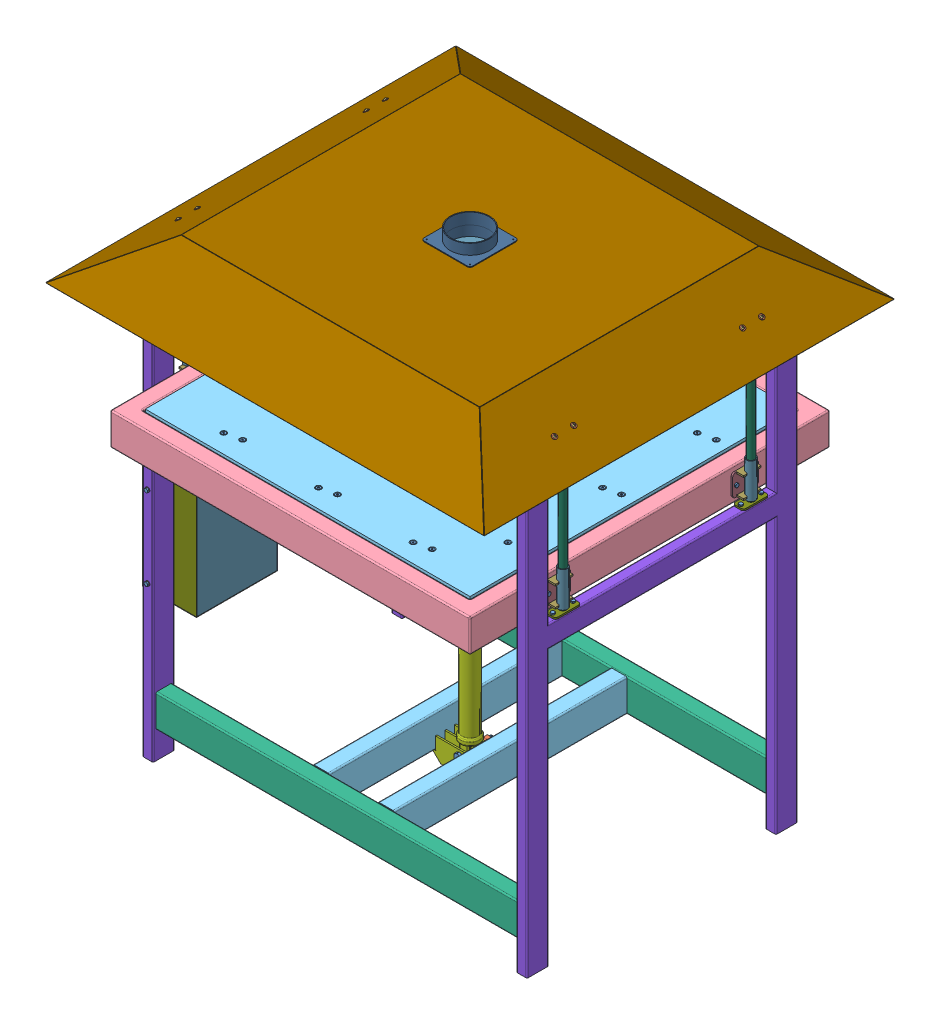
SolidWorks assembly SPR-V1 0000.00-A Sheetpress assembly, configuration Default. Lengths in mm. (continued)
Components (placement in the parent): (continued)
- Extraction hood^SPR-V1 0000.00-A Sheetpress assembly-1: Extraction hood^SPR-V1 0000.00-A Sheetpress assembly [Default] at origin size (1620.39 205.36 1515.92) (virtual)
  - SPR-V1 0000.02-A Hood-1: SPR-V1 0000.02-A Hood [Default] at (0 140 0) x (1 0 0) z (0 1 0) size (1620.39 1515.92 163.86)
  - SPR-V1 02 Extraction fitting-1: SPR-V1 02 Extraction fitting [Default] at (0 244.5 0) size (180 80 180)
  - plain washer large grade ac_iso-1: plain washer large grade ac_iso [Washer ISO 7093 - 6] at (694.9392 153.5499 -383) x (-0.529105 -0.848557 0) z (0 0 1) size (1.6 18 18)
  - plain washer large grade ac_iso-2: plain washer large grade ac_iso [Washer ISO 7093 - 6] at (694.9392 153.5499 -312) x (-0.529105 -0.848557 0) z (0 0 1) size (1.6 18 18)
  - plain washer large grade ac_iso-3: plain washer large grade ac_iso [Washer ISO 7093 - 6] at (694.9392 153.5499 312) x (-0.529105 -0.848557 0) z (0 0 1) size (1.6 18 18)
  - plain washer large grade ac_iso-4: plain washer large grade ac_iso [Washer ISO 7093 - 6] at (694.9392 153.5499 383) x (-0.529105 -0.848557 0) z (0 0 1) size (1.6 18 18)
  - plain washer large grade ac_iso-5: plain washer large grade ac_iso [Washer ISO 7093 - 6] at (-694.9392 153.5499 -383) x (0.529105 -0.848557 0) z (0 0 1) size (1.6 18 18)
  - plain washer large grade ac_iso-6: plain washer large grade ac_iso [Washer ISO 7093 - 6] at (-694.9392 153.5499 312) x (0.529105 -0.848557 0) z (0 0 1) size (1.6 18 18)
  - plain washer large grade ac_iso-7: plain washer large grade ac_iso [Washer ISO 7093 - 6] at (-694.9392 153.5499 383) x (0.529105 -0.848557 0) z (0 0 1) size (1.6 18 18)
  - socket button head screw_iso-1: socket button head screw_iso [ISO 7380 - M6 x 12 - 12N] at (-697.5318 157.7078 383) x (0.529105 -0.848557 0) z (0 0 1) size (15.3 10.5 10.5)
  - socket button head screw_iso-2: socket button head screw_iso [ISO 7380 - M6 x 12 - 12N] at (-697.5318 157.7078 312) x (0.529105 -0.848557 0) z (0 0 1) size (15.3 10.5 10.5)
  - socket button head screw_iso-3: socket button head screw_iso [ISO 7380 - M6 x 12 - 12N] at (-697.5318 157.7078 -383) x (0.529105 -0.848557 0) z (0 0 1) size (15.3 10.5 10.5)
  - socket button head screw_iso-4: socket button head screw_iso [ISO 7380 - M6 x 12 - 12N] at (-697.5318 157.7078 -312) x (0.529105 -0.848557 0) z (0 0 1) size (15.3 10.5 10.5)
  - socket button head screw_iso-5: socket button head screw_iso [ISO 7380 - M6 x 12 - 12N] at (697.5318 157.7078 -312) x (-0.529105 -0.848557 0) z (0 0 1) size (15.3 10.5 10.5)
  - socket button head screw_iso-6: socket button head screw_iso [ISO 7380 - M6 x 12 - 12N] at (697.5318 157.7078 -383) x (-0.529105 -0.848557 0) z (0 0 1) size (15.3 10.5 10.5)
  - socket button head screw_iso-7: socket button head screw_iso [ISO 7380 - M6 x 12 - 12N] at (697.5318 157.7078 383) x (-0.529105 -0.848557 0) z (0 0 1) size (15.3 10.5 10.5)
  - socket button head screw_iso-8: socket button head screw_iso [ISO 7380 - M6 x 12 - 12N] at (697.5318 157.7078 312) x (-0.529105 -0.848557 0) z (0 0 1) size (15.3 10.5 10.5)
  - plain washer large grade ac_iso-8: plain washer large grade ac_iso [Washer ISO 7093 - 6] at (-694.9392 153.5499 -312) x (0.529105 -0.848557 0) z (0 0 1) size (1.6 18 18)
- Electronics enclosure^SPR-V1 0000.00-A Sheetpress assembly-1: Electronics enclosure^SPR-V1 0000.00-A Sheetpress assembly [Default] at origin size (223.77 526.27 386.9) (virtual)
  - SPR-V1 5000.01-A Electronics Enclosure Front 496x296 2mm Sheet Steel-1: SPR-V1 5000.01-A Electronics Enclosure Front 496x296 2mm Sheet Steel [Default] at (-791 -800 270) x (0 0 -1) z (1 0 0) size (296 496 2)
  - SPR-V1 5000.01-A Electronics Enclosure Bottom 300x200 2mm Sheet Steel-1: SPR-V1 5000.01-A Electronics Enclosure Bottom 300x200 2mm Sheet Steel [Default] at (-691 -1050 270) x (0 0 -1) z (0 1 0) size (300 200 2)
  - SPR-V1 5000.02-A-A Front Panel Mount Tab 6mm Sheet Steel-1: SPR-V1 5000.02-A-A Front Panel Mount Tab 6mm Sheet Steel [Default] at (-789 -1048 418) x (0 0 -1) z (0 -1 0) size (35.76 6 35.76)
  - SPR-V1 5000.02-A-A Front Panel Mount Tab 6mm Sheet Steel-2: SPR-V1 5000.02-A-A Front Panel Mount Tab 6mm Sheet Steel [Default] at (-783 -1048 122) x (0 0 1) z (0 -1 0) size (35.76 6 35.76)
  - SPR-V1 5000.02-A-A Front Panel Mount Tab 6mm Sheet Steel-3: SPR-V1 5000.02-A-A Front Panel Mount Tab 6mm Sheet Steel [Default] at (-783 -552 122) x (0 -1 0) z (0 0 -1) size (35.76 6 35.76)
  - SPR-V1 5000.02-A-A Front Panel Mount Tab 6mm Sheet Steel-4: SPR-V1 5000.02-A-A Front Panel Mount Tab 6mm Sheet Steel [Default] at (-783 -552 418) x (0 0 -1) z (0 1 0) size (35.76 6 35.76)
  - SPR-V1 5000.01-A Electronics Enclosure Back 496x296 2mm Sheet Steel-1: SPR-V1 5000.01-A Electronics Enclosure Back 496x296 2mm Sheet Steel [Default] at (-593 -830.6979 333.9633) x (0 0 -1) z (1 0 0) size (296 496 2)
  - SPR-V1 5000.01-A Electronics Enclosure Top 300x200 2mm Sheet Steel-1: SPR-V1 5000.01-A Electronics Enclosure Top 300x200 2mm Sheet Steel [Default] at (-691 -550 270) x (0 0 -1) z (0 -1 0) size (300 200 2)
  - SPR-V1 5000.01-A Electronics Enclosure Right 496x200mm Sheet Steel-1: SPR-V1 5000.01-A Electronics Enclosure Right 496x200mm Sheet Steel [Default] at (-691 -800 418) size (200 496 2)
  - SPR-V1 5000.01-A Electronics Enclosure Left 496x200mm Sheet Steel-1: SPR-V1 5000.01-A Electronics Enclosure Left 496x200mm Sheet Steel [Default] at (-691 -800 120) size (200 496 2)
  - SPR-V1 5000.00-A REX C1000 PID Controler-1: SPR-V1 5000.00-A REX C1000 PID Controler [Default] at (-798.9248 -676.7129 172.0859) x (0 0 1) z (-1 0 0) size (47.83 47.57 107.37)
  - SPR-V1 5000.00-A REX C1000 PID Controler-2: SPR-V1 5000.00-A REX C1000 PID Controler [Default] at (-798.9248 -577.7129 172.0859) x (0 0 1) z (-1 0 0) size (47.83 47.57 107.37)
  - SPR-V1 5000.00-A Rotary Switch-1: SPR-V1 5000.00-A Rotary Switch [Default] at (-732.7739 -599.9141 313.1392) x (0 0 1) z (-1 0 0) size (48 48 55.77)
  - SPR-V1 5000.00-A Emergency Stop-1: SPR-V1 5000.00-A Emergency Stop [Défaut] at (-743 -700.5 344) x (0 0 -1) z (-1 0 0) size (40 40 71)
  - SPR-V1 14 M25 Cable Gland-1: SPR-V1 14 M25 Cable Gland [M20] at (-691.0017 -1032.6252 180.0036) x (-0.837169 0 -0.546944) z (-0.546944 0 0.837169) size (33.12 53.02 29.38)
  - SPR-V1 14 M25 Cable Gland-2: SPR-V1 14 M25 Cable Gland [M20] at (-691.0017 -1032.6252 240.0036) x (-0.837169 0 -0.546944) z (-0.546944 0 0.837169) size (33.12 53.02 29.38)
  - SPR-V1 14 M25 Cable Gland-3: SPR-V1 14 M25 Cable Gland [M20] at (-691.0017 -1032.6252 300.0036) x (-0.837169 0 -0.546944) z (-0.546944 0 0.837169) size (33.12 53.02 29.38)
  - SPR-V1 16 M10 Gland-1: SPR-V1 16 M10 Gland [M20] at (-691.0071 -1031.8322 359.9966) x (-0.546944 0 0.837169) z (0.837169 0 0.546944) size (13.25 53.02 11.75)
  - plain washer large grade ac_iso-1: plain washer large grade ac_iso [Washer ISO 7093 - 6] at (-791 -562 132) size (1.6 18 18)
  - plain washer large grade ac_iso-2: plain washer large grade ac_iso [Washer ISO 7093 - 6] at (-791 -562 408) size (1.6 18 18)
  - plain washer large grade ac_iso-3: plain washer large grade ac_iso [Washer ISO 7093 - 6] at (-791 -1038 132) size (1.6 18 18)
  - plain washer large grade ac_iso-4: plain washer large grade ac_iso [Washer ISO 7093 - 6] at (-791 -1038 408) size (1.6 18 18)
  - socket button head screw_iso-1: socket button head screw_iso [ISO 7380 - M6 x 12 - 12N] at (-795.9 -1038 408) size (15.3 10.5 10.5)
  - socket button head screw_iso-2: socket button head screw_iso [ISO 7380 - M6 x 12 - 12N] at (-795.9 -1038 132) size (15.3 10.5 10.5)
  - socket button head screw_iso-3: socket button head screw_iso [ISO 7380 - M6 x 12 - 12N] at (-795.9 -562 408) size (15.3 10.5 10.5)
  - socket button head screw_iso-4: socket button head screw_iso [ISO 7380 - M6 x 12 - 12N] at (-795.9 -562 132) size (15.3 10.5 10.5)
  - plain washer normal grade a_iso-1: plain washer normal grade a_iso [Washer ISO 7089 - 8] at (-691 -650 418) x (0 0 1) z (-1 0 0) size (1.6 16 16)
  - plain washer normal grade a_iso-2: plain washer normal grade a_iso [Washer ISO 7089 - 8] at (-691 -650 501.6) x (0 0 1) z (-1 0 0) size (1.6 16 16)
  - plain washer normal grade a_iso-3: plain washer normal grade a_iso [Washer ISO 7089 - 8] at (-691 -950 418) x (0 0 1) z (-1 0 0) size (1.6 16 16)
  - plain washer normal grade a_iso-4: plain washer normal grade a_iso [Washer ISO 7089 - 8] at (-691 -950 501.6) x (0 0 1) z (-1 0 0) size (1.6 16 16)
  - hex bolt gradeab_iso-1: hex bolt gradeab_iso [ISO 4014 - M8 x 100 x 100-N] at (-691 -650 506.9) x (0 0 -1) z (1 0 0) size (105.3 15.01 13)
  - hex bolt gradeab_iso-2: hex bolt gradeab_iso [ISO 4014 - M8 x 100 x 100-N] at (-691 -950 506.9) x (0 0 -1) z (1 0 0) size (105.3 15.01 13)
  - hex nut gradec_iso-1: hex nut gradec_iso [ISO - 4034 - M8 - N] at (-691 -650 408.5) x (0.923728 0.383049 0) z (0 0 -1) size (13 15.01 7.9)
  - hex nut gradec_iso-2: hex nut gradec_iso [ISO - 4034 - M8 - N] at (-691 -950 408.5) x (0.923728 0.383049 0) z (0 0 -1) size (13 15.01 7.9)
Mates (geometry in assembly coordinates):
- Coincident64: coincident: plane of plain washer normal grade a_iso-1 through (-714 95 350) normal (-1 0 0); plane of hex bolt gradeab_iso-1 through (-714 93.8564 350) normal (1 0 0)
- Coincident65: coincident: plane of plain washer normal grade a_iso-3 through (-714 95 -350) normal (-1 0 0); plane of hex bolt gradeab_iso-2 through (-714 93.8564 -350) normal (1 0 0)
- Coincident66: coincident: plane of plain washer normal grade a_iso-2 through (-714 95 0) normal (-1 0 0); plane of hex bolt gradeab_iso-3 through (-714 93.8564 0) normal (1 0 0)
- Coincident67: coincident: plane of plain washer normal grade a_iso-9 through (714 74.2723 -336.1366) normal (1 0 0); plane of hex bolt gradeab_iso-4 through (714 74.7089 -337.1936) normal (-1 0 0)
- Coincident68: coincident: plane of plain washer normal grade a_iso-8 through (714 74.2723 13.8634) normal (1 0 0); plane of hex bolt gradeab_iso-5 through (714 74.7089 12.8064) normal (-1 0 0)
- Coincident69: coincident: plane of plain washer normal grade a_iso-7 through (714 74.2723 363.8634) normal (1 0 0); plane of hex bolt gradeab_iso-6 through (714 74.7089 362.8064) normal (-1 0 0)
- Concentric122: concentric: cylinder of plain washer normal grade a_iso-12 through (-570.075 80 -350) axis (1 0 0) radius 8.5; cylinder of hex nut gradec_iso-130 through (-611.1375 80 -350) axis (1 0 0) radius 8
- Coincident150: coincident: plane of plain washer normal grade a_iso-12 through (-602 74.2723 -336.1366) normal (1 0 0); plane of hex nut gradec_iso-130 through (-602 80 -326) normal (-1 0 0)
- Concentric123: concentric: cylinder of plain washer normal grade a_iso-11 through (-570.075 80 0) axis (1 0 0) radius 8.5; cylinder of hex nut gradec_iso-131 through (-619.1375 80 0) axis (1 0 0) radius 4
- Coincident151: coincident: plane of plain washer normal grade a_iso-11 through (-602 74.2723 13.8634) normal (1 0 0); plane of hex nut gradec_iso-131 through (-602 87.5056 0) normal (-1 0 0)
- Concentric124: concentric: cylinder of plain washer normal grade a_iso-10 through (-570.075 80 350) axis (1 0 0) radius 8.5; cylinder of hex nut gradec_iso-132 through (-611.1375 80 350) axis (1 0 0) radius 8
- Coincident152: coincident: plane of plain washer normal grade a_iso-10 through (-602 74.2723 363.8634) normal (1 0 0); plane of hex nut gradec_iso-132 through (-602 80 374) normal (-1 0 0)
- Concentric125: concentric: cylinder of plain washer normal grade a_iso-4 through (570.075 80 350) axis (-1 0 0) radius 8.5; cylinder of hex nut gradec_iso-133 through (611.1375 80 350) axis (-1 0 0) radius 8
- Coincident153: coincident: plane of plain washer normal grade a_iso-4 through (602 95 350) normal (-1 0 0); plane of hex nut gradec_iso-133 through (602 80 326) normal (1 0 0)
- Concentric126: concentric: cylinder of plain washer normal grade a_iso-6 through (570.075 80 -350) axis (-1 0 0) radius 8.5; cylinder of hex nut gradec_iso-134 through (611.1375 80 -350) axis (-1 0 0) radius 8
- Coincident154: coincident: plane of plain washer normal grade a_iso-6 through (602 95 -350) normal (-1 0 0); plane of hex nut gradec_iso-134 through (602 80 -374) normal (1 0 0)
- Concentric127: concentric: cylinder of plain washer normal grade a_iso-5 through (570.075 80 0) axis (-1 0 0) radius 8.5; cylinder of hex nut gradec_iso-135 through (619.1375 80 0) axis (-1 0 0) radius 4
- Coincident155: coincident: plane of plain washer normal grade a_iso-5 through (602 95 0) normal (-1 0 0); plane of hex nut gradec_iso-135 through (602 87.5056 0) normal (1 0 0)
- Concentric129: concentric: cone of hex nut gradec_iso-136 through (0 -1389 -53.9) axis (0 0 -1); cylinder of hex nut gradec_iso-137 through (0 -1389 -44.7625) axis (0 0 -1) radius 8
- Coincident157: coincident: plane of hex nut gradec_iso-136 through (-22.1695 -1398.1932 -53.9) normal (0 0 -1); plane of hex nut gradec_iso-137 through (-22.1695 -1398.1932 -53.9) normal (0 0 1)
- Concentric133: concentric: cylinder of hex nut gradec_iso-140 through (-64.58 -546.9999 -64.5798) axis (0.707107 0 0.707107) radius 959.9311; cylinder of hex nut gradec_iso-141 through (-58.6634 -546.9999 -58.6633) axis (-0.707107 0 -0.707107) radius 8
- Coincident160: coincident: plane of hex nut gradec_iso-140 through (-48.154 -546.9999 -82.095) normal (-0.707107 0 -0.707107); plane of hex nut gradec_iso-141 through (-48.1546 -546.8137 -82.0945) normal (0.707107 0 0.707107)
- Distance8: distance = 10 mm: plane of hex bolt gradeab_iso-10 through (-83.4387 -546.9999 -83.4385) normal (-0.707107 0 -0.707107); plane of hex nut gradec_iso-141 through (-59.3975 -546.8137 -93.3375) normal (-0.707107 0 -0.707107)
- Concentric905: concentric: cylinder of Frame^SPR-V1 0000.00-A Sheetpress assembly-1/SPR-V1 0000.01-A Jack mount lower-1 through (0 -1389 32) axis (0 0 1) radius 9; cylinder of hex bolt gradeab_iso-8 through (0 -1389 48) axis (0 0 1) radius 12
- Coincident365: coincident: plane of Frame^SPR-V1 0000.00-A Sheetpress assembly-1/SPR-V1 0000.01-A Jack mount lower-1 through (0 0 38) normal (0 0 1); plane of hex bolt gradeab_iso-8 through (0 -1375.1436 38) normal (0 0 -1)
- Concentric906: concentric: cylinder of Frame^SPR-V1 0000.00-A Sheetpress assembly-1/SPR-V1 1000.01-A Side frame-1 through (671 80 350) axis (1 0 0) radius 9; cylinder of plain washer normal grade a_iso-7 through (745.925 80 350) axis (1 0 0) radius 8.5
- Coincident366: coincident: plane of Frame^SPR-V1 0000.00-A Sheetpress assembly-1/SPR-V1 1000.01-A Side frame-1 through (711 0 0) normal (1 0 0); plane of plain washer normal grade a_iso-7 through (711 76.7543 357.8559) normal (-1 0 0)
- Concentric907: concentric: cylinder of Frame^SPR-V1 0000.00-A Sheetpress assembly-1/SPR-V1 1000.01-A Side frame-1 through (671 80 0) axis (1 0 0) radius 9; cylinder of plain washer normal grade a_iso-8 through (745.925 80 0) axis (1 0 0) radius 8.5
- Coincident367: coincident: plane of Frame^SPR-V1 0000.00-A Sheetpress assembly-1/SPR-V1 1000.01-A Side frame-1 through (711 0 0) normal (1 0 0); plane of plain washer normal grade a_iso-8 through (711 76.7543 7.8559) normal (-1 0 0)
- Concentric908: concentric: cylinder of Frame^SPR-V1 0000.00-A Sheetpress assembly-1/SPR-V1 1000.01-A Side frame-1 through (671 80 -350) axis (1 0 0) radius 9; cylinder of plain washer normal grade a_iso-9 through (745.925 80 -350) axis (1 0 0) radius 8.5
- Coincident368: coincident: plane of Frame^SPR-V1 0000.00-A Sheetpress assembly-1/SPR-V1 1000.01-A Side frame-1 through (711 0 0) normal (1 0 0); plane of plain washer normal grade a_iso-9 through (711 76.7543 -342.1441) normal (-1 0 0)
- Concentric909: concentric: cylinder of Frame^SPR-V1 0000.00-A Sheetpress assembly-1/SPR-V1 1000.01-A Side frame-1 through (671 80 -350) axis (1 0 0) radius 9; cylinder of hex bolt gradeab_iso-4 through (724 80 -350) axis (1 0 0) radius 12
- Concentric910: concentric: cylinder of Frame^SPR-V1 0000.00-A Sheetpress assembly-1/SPR-V1 1000.01-A Side frame-1 through (671 80 0) axis (1 0 0) radius 9; cylinder of hex bolt gradeab_iso-5 through (724 80 0) axis (1 0 0) radius 12
- Concentric911: concentric: cylinder of Frame^SPR-V1 0000.00-A Sheetpress assembly-1/SPR-V1 1000.01-A Side frame-1 through (671 80 350) axis (1 0 0) radius 9; cylinder of hex bolt gradeab_iso-6 through (724 80 350) axis (1 0 0) radius 12
- Concentric916: concentric: cylinder of Frame^SPR-V1 0000.00-A Sheetpress assembly-1/SPR-V1 1000.01-A Side frame-2 through (-711 80 350) axis (1 0 0) radius 9; cylinder of plain washer normal grade a_iso-1 through (-745.925 80 350) axis (-1 0 0) radius 8.5
- Coincident373: coincident: plane of Frame^SPR-V1 0000.00-A Sheetpress assembly-1/SPR-V1 1000.01-A Side frame-2 through (-711 0 0) normal (-1 0 0); plane of plain washer normal grade a_iso-1 through (-711 88.5 350) normal (1 0 0)
- Concentric917: concentric: cylinder of Frame^SPR-V1 0000.00-A Sheetpress assembly-1/SPR-V1 1000.01-A Side frame-2 through (-711 80 0) axis (1 0 0) radius 9; cylinder of plain washer normal grade a_iso-2 through (-745.925 80 0) axis (-1 0 0) radius 8.5
- Coincident374: coincident: plane of Frame^SPR-V1 0000.00-A Sheetpress assembly-1/SPR-V1 1000.01-A Side frame-2 through (-711 0 0) normal (-1 0 0); plane of plain washer normal grade a_iso-2 through (-711 88.5 0) normal (1 0 0)
- Concentric918: concentric: cylinder of Frame^SPR-V1 0000.00-A Sheetpress assembly-1/SPR-V1 1000.01-A Side frame-2 through (-711 80 -350) axis (1 0 0) radius 9; cylinder of plain washer normal grade a_iso-3 through (-745.925 80 -350) axis (-1 0 0) radius 8.5
- Coincident375: coincident: plane of Frame^SPR-V1 0000.00-A Sheetpress assembly-1/SPR-V1 1000.01-A Side frame-2 through (-711 0 0) normal (-1 0 0); plane of plain washer normal grade a_iso-3 through (-711 88.5 -350) normal (1 0 0)
- Concentric919: concentric: cylinder of Frame^SPR-V1 0000.00-A Sheetpress assembly-1/SPR-V1 1000.01-A Side frame-2 through (-711 80 350) axis (1 0 0) radius 9; cylinder of hex bolt gradeab_iso-1 through (-724 80 350) axis (-1 0 0) radius 12
- Concentric920: concentric: cylinder of Frame^SPR-V1 0000.00-A Sheetpress assembly-1/SPR-V1 1000.01-A Side frame-2 through (-711 80 -350) axis (1 0 0) radius 9; cylinder of hex bolt gradeab_iso-2 through (-724 80 -350) axis (-1 0 0) radius 12
- Concentric921: concentric: cylinder of Frame^SPR-V1 0000.00-A Sheetpress assembly-1/SPR-V1 1000.01-A Side frame-2 through (-711 80 0) axis (1 0 0) radius 9; cylinder of hex bolt gradeab_iso-3 through (-724 80 0) axis (-1 0 0) radius 12
- Concentric926: concentric: cylinder of Frame^SPR-V1 0000.00-A Sheetpress assembly-1/SPR-V1 0000.01-A Jack mount lower-2 through (0 -1389 -38) axis (0 0 1) radius 9; cylinder of hex nut gradec_iso-136 through (0 -1389 -28.8625) axis (0 0 -1) radius 8
- Coincident383: coincident: plane of Frame^SPR-V1 0000.00-A Sheetpress assembly-1/SPR-V1 0000.01-A Jack mount lower-2 through (0 0 -38) normal (0 0 -1); plane of hex nut gradec_iso-136 through (-22.1695 -1398.1932 -38) normal (0 0 1)
- Concentric958: concentric: cylinder of Pressing plate upper^SPR-V1 0000.00-A Sheetpress assembly-2/SPR-V1 2100.01-A Pressing plate frame upper-1 through (-665 80 350) axis (1 0 0) radius 9; cylinder of plain washer normal grade a_iso-4 through (570.075 80 350) axis (-1 0 0) radius 8.5
- Coincident409: coincident: plane of Pressing plate upper^SPR-V1 0000.00-A Sheetpress assembly-2/SPR-V1 2100.01-A Pressing plate frame upper-1 through (605 120 -605) normal (-1 0 0); plane of plain washer normal grade a_iso-4 through (605 88.5 350) normal (1 0 0)
- Concentric959: concentric: cylinder of Pressing plate upper^SPR-V1 0000.00-A Sheetpress assembly-2/SPR-V1 2100.01-A Pressing plate frame upper-1 through (-665 80 0) axis (1 0 0) radius 9; cylinder of plain washer normal grade a_iso-5 through (570.075 80 0) axis (-1 0 0) radius 8.5
- Coincident410: coincident: plane of Pressing plate upper^SPR-V1 0000.00-A Sheetpress assembly-2/SPR-V1 2100.01-A Pressing plate frame upper-1 through (605 120 -605) normal (-1 0 0); plane of plain washer normal grade a_iso-5 through (605 88.5 0) normal (1 0 0)
- Concentric960: concentric: cylinder of Pressing plate upper^SPR-V1 0000.00-A Sheetpress assembly-2/SPR-V1 2100.01-A Pressing plate frame upper-1 through (-665 80 -350) axis (1 0 0) radius 9; cylinder of plain washer normal grade a_iso-6 through (570.075 80 -350) axis (-1 0 0) radius 8.5
- Coincident411: coincident: plane of Pressing plate upper^SPR-V1 0000.00-A Sheetpress assembly-2/SPR-V1 2100.01-A Pressing plate frame upper-1 through (605 120 -605) normal (-1 0 0); plane of plain washer normal grade a_iso-6 through (605 88.5 -350) normal (1 0 0)
- Concentric961: concentric: cylinder of Pressing plate upper^SPR-V1 0000.00-A Sheetpress assembly-2/SPR-V1 2100.01-A Pressing plate frame upper-1 through (-665 80 350) axis (1 0 0) radius 9; cylinder of plain washer normal grade a_iso-10 through (-570.075 80 350) axis (1 0 0) radius 8.5
- Coincident412: coincident: plane of Pressing plate upper^SPR-V1 0000.00-A Sheetpress assembly-2/SPR-V1 2100.01-A Pressing plate frame upper-1 through (-605 120 -605) normal (1 0 0); plane of plain washer normal grade a_iso-10 through (-605 76.7543 357.8559) normal (-1 0 0)
- Concentric962: concentric: cylinder of Pressing plate upper^SPR-V1 0000.00-A Sheetpress assembly-2/SPR-V1 2100.01-A Pressing plate frame upper-1 through (-665 80 0) axis (1 0 0) radius 9; cylinder of plain washer normal grade a_iso-11 through (-570.075 80 0) axis (1 0 0) radius 8.5
- Coincident413: coincident: plane of Pressing plate upper^SPR-V1 0000.00-A Sheetpress assembly-2/SPR-V1 2100.01-A Pressing plate frame upper-1 through (-605 120 -605) normal (1 0 0); plane of plain washer normal grade a_iso-11 through (-605 76.7543 7.8559) normal (-1 0 0)
- Concentric963: concentric: cylinder of Pressing plate upper^SPR-V1 0000.00-A Sheetpress assembly-2/SPR-V1 2100.01-A Pressing plate frame upper-1 through (-665 80 -350) axis (1 0 0) radius 9; cylinder of plain washer normal grade a_iso-12 through (-570.075 80 -350) axis (1 0 0) radius 8.5
- Coincident414: coincident: plane of Pressing plate upper^SPR-V1 0000.00-A Sheetpress assembly-2/SPR-V1 2100.01-A Pressing plate frame upper-1 through (-605 120 -605) normal (1 0 0); plane of plain washer normal grade a_iso-12 through (-605 76.7543 -342.1441) normal (-1 0 0)
- Distance21: distance = 300 mm: plane of Pressing plate lower^SPR-V1 0000.00-A Sheetpress assembly-1/SPR-V1 3100.01-A Pressing plate frame lower-1 through (0 -300 0) normal (0 1 0); plane of Pressing plate upper^SPR-V1 0000.00-A Sheetpress assembly-2/SPR-V1 2100.01-A Pressing plate frame upper-1 through (0 0 0) normal (0 -1 0)
- Parallel20: parallel: plane of Pressing plate lower^SPR-V1 0000.00-A Sheetpress assembly-1/SPR-V1 3100.03-A Pressing plate support structure lower A-1 through (0 -307 0) normal (0 -1 0); plane of assembly through (0 0 0) normal (0 1 0)
- Coincident423: coincident: plane of Pressing plate lower^SPR-V1 0000.00-A Sheetpress assembly-1/SPR-V1 3100.03-A Pressing plate support structure lower A-1 through (0 -307 0) normal (0 0 1); plane of assembly through (0 0 0) normal (0 0 1)
- Coincident424: coincident: plane of Pressing plate lower^SPR-V1 0000.00-A Sheetpress assembly-1/SPR-V1 3100.03-A Pressing plate support structure lower A-1 through (0 -307 0) normal (-1 0 0); plane of assembly through (0 0 0) normal (1 0 0)
- Parallel21: parallel: plane of Pressing plate lower^SPR-V1 0000.00-A Sheetpress assembly-1/SPR-V1 3100.03-A Pressing plate support structure lower B-1 through (0 -307 0) normal (0 -1 0); plane of assembly through (0 0 0) normal (0 1 0)
- Coincident425: coincident: plane of Pressing plate lower^SPR-V1 0000.00-A Sheetpress assembly-1/SPR-V1 3100.03-A Pressing plate support structure lower B-1 through (0 -307 0) normal (-1 0 0); plane of assembly through (0 0 0) normal (1 0 0)
- Coincident426: coincident: plane of Pressing plate lower^SPR-V1 0000.00-A Sheetpress assembly-1/SPR-V1 3100.03-A Pressing plate support structure lower B-1 through (0 -307 0) normal (0 0 -1); plane of assembly through (0 0 0) normal (0 0 1)
- Concentric972: concentric: cylinder of Pressing plate lower^SPR-V1 0000.00-A Sheetpress assembly-1/SPR-V1 3100.03-A Jack mount-1 through (72.6178 -546.9999 72.6179) axis (-0.707107 0 -0.707107) radius 9; cylinder of hex nut gradec_iso-140 through (-47.4204 -546.9999 -47.4203) axis (-0.707107 0 -0.707107) radius 8
- Concentric973: concentric: cylinder of Pressing plate lower^SPR-V1 0000.00-A Sheetpress assembly-1/SPR-V1 3100.03-A Jack mount-2 through (99.4878 -546.9999 99.488) axis (-0.707107 0 -0.707107) radius 9; cylinder of hex bolt gradeab_iso-10 through (22.6273 -546.9999 22.6275) axis (0.707107 0 0.707107) radius 12
- Coincident427: coincident: plane of Pressing plate lower^SPR-V1 0000.00-A Sheetpress assembly-1/SPR-V1 3100.03-A Jack mount-2 through (620.5563 -307 -589.4437) normal (0.707107 0 0.707107); plane of hex bolt gradeab_iso-10 through (15.5563 -533.1435 15.5564) normal (-0.707107 0 -0.707107)
- Coincident429: coincident: line of Pressing mechanism^SPR-V1 0000.00-A Sheetpress assembly-1/SPR-V1 4000.01-A Spring sleeve-1 through (0 -766 17) axis (0 0 -1)
- Distance25: distance = 20 mm: plane of Pressing plate lower^SPR-V1 0000.00-A Sheetpress assembly-1/SPR-V1 3100.03-A Pressing plate support structure lower B-1 through (-19.0919 -527 -23.3345) normal (0 -1 0); point of Pressing mechanism^SPR-V1 0000.00-A Sheetpress assembly-1/SPR-V1 4000.02-A Spring rod-1
- Parallel26: parallel: plane of Pressing plate lower^SPR-V1 0000.00-A Sheetpress assembly-1/SPR-V1 3100.03-A Pressing plate support structure lower B-1 through (-605 -407 -600.7574) normal (-0.707107 0 0.707107); line of Pressing mechanism^SPR-V1 0000.00-A Sheetpress assembly-1/SPR-V1 4000.02-A Spring rod-1 through (9.5459 -547 9.5459) axis (-0.707107 0 -0.707107)
- Parallel27: parallel: plane of Pressing mechanism^SPR-V1 0000.00-A Sheetpress assembly-1/SPR-V1 15 Die Spring-1 through (0 -719.4 26.5625) normal (1 0 0); plane of assembly through (0 0 0) normal (1 0 0)
- Parallel28: parallel: plane of Pressing mechanism^SPR-V1 0000.00-A Sheetpress assembly-1/SPR-V1 01 Cylinder-1 through (-17.5 -1404 24) normal (0 0 1); plane of assembly through (0 0 0) normal (0 0 1)
- Distance26: distance = 1389 mm: unknown of Pressing mechanism^SPR-V1 0000.00-A Sheetpress assembly-1/SPR-V1 01 Cylinder-1
- Coincident433: coincident: plane of Frame^SPR-V1 0000.00-A Sheetpress assembly-1/SPR-V1 1000.01-A Side frame-2 through (-671 0 420) normal (0 0 -1); plane of Electronics enclosure^SPR-V1 0000.00-A Sheetpress assembly-1/SPR-V1 5000.01-A Electronics Enclosure Right 496x200mm Sheet Steel-1 through (-691 -800 420) normal (0 0 1)
- Coincident434: coincident: plane of Frame^SPR-V1 0000.00-A Sheetpress assembly-1/SPR-V1 1000.01-A Side frame-2 through (-671 0 500) normal (0 0 1); plane of Electronics enclosure^SPR-V1 0000.00-A Sheetpress assembly-1/plain washer normal grade a_iso-2 through (-691 -642 500) normal (0 0 -1)
- Coincident435: coincident: plane of Frame^SPR-V1 0000.00-A Sheetpress assembly-1/SPR-V1 1000.01-A Side frame-2 through (-671 0 500) normal (0 0 1); plane of Electronics enclosure^SPR-V1 0000.00-A Sheetpress assembly-1/plain washer normal grade a_iso-4 through (-691 -942 500) normal (0 0 -1)
- Concentric1011: concentric: cylinder of Pressing plate lower^SPR-V1 0000.00-A Sheetpress assembly-1/SPR-V1 3100.01-A Pressing plate frame lower-1 through (-665 -360 -383) axis (1 0 0) radius 5; cylinder of Sliding mechanism^SPR-V1 0000.00-A Sheetpress assembly-1/plain washer normal grade a_iso-1 through (570.075 -360 -383) axis (-1 0 0) radius 4.2
- Coincident469: coincident: plane of Pressing plate lower^SPR-V1 0000.00-A Sheetpress assembly-1/SPR-V1 3100.01-A Pressing plate frame lower-1 through (605 -420 -605) normal (-1 0 0); plane of Sliding mechanism^SPR-V1 0000.00-A Sheetpress assembly-1/plain washer normal grade a_iso-1 through (605 -355.8 -383) normal (1 0 0)
- Concentric1012: concentric: cylinder of Pressing plate lower^SPR-V1 0000.00-A Sheetpress assembly-1/SPR-V1 3100.01-A Pressing plate frame lower-1 through (-665 -360 -312) axis (1 0 0) radius 5; cylinder of Sliding mechanism^SPR-V1 0000.00-A Sheetpress assembly-1/plain washer normal grade a_iso-2 through (570.075 -360 -312) axis (-1 0 0) radius 4.2
- Coincident470: coincident: plane of Pressing plate lower^SPR-V1 0000.00-A Sheetpress assembly-1/SPR-V1 3100.01-A Pressing plate frame lower-1 through (605 -420 -605) normal (-1 0 0); plane of Sliding mechanism^SPR-V1 0000.00-A Sheetpress assembly-1/plain washer normal grade a_iso-2 through (605 -355.8 -312) normal (1 0 0)
- Concentric1013: concentric: cylinder of Pressing plate lower^SPR-V1 0000.00-A Sheetpress assembly-1/SPR-V1 3100.01-A Pressing plate frame lower-1 through (-665 -360 312) axis (1 0 0) radius 5; cylinder of Sliding mechanism^SPR-V1 0000.00-A Sheetpress assembly-1/plain washer normal grade a_iso-3 through (570.075 -360 312) axis (-1 0 0) radius 4.2
- Coincident471: coincident: plane of Pressing plate lower^SPR-V1 0000.00-A Sheetpress assembly-1/SPR-V1 3100.01-A Pressing plate frame lower-1 through (605 -420 -605) normal (-1 0 0); plane of Sliding mechanism^SPR-V1 0000.00-A Sheetpress assembly-1/plain washer normal grade a_iso-3 through (605 -355.8 312) normal (1 0 0)
- Concentric1014: concentric: cylinder of Pressing plate lower^SPR-V1 0000.00-A Sheetpress assembly-1/SPR-V1 3100.01-A Pressing plate frame lower-1 through (-665 -360 383) axis (1 0 0) radius 5; cylinder of Sliding mechanism^SPR-V1 0000.00-A Sheetpress assembly-1/plain washer normal grade a_iso-4 through (570.075 -360 383) axis (-1 0 0) radius 4.2
- Coincident472: coincident: plane of Pressing plate lower^SPR-V1 0000.00-A Sheetpress assembly-1/SPR-V1 3100.01-A Pressing plate frame lower-1 through (605 -420 -605) normal (-1 0 0); plane of Sliding mechanism^SPR-V1 0000.00-A Sheetpress assembly-1/plain washer normal grade a_iso-4 through (605 -355.8 383) normal (1 0 0)
- Concentric1015: concentric: cylinder of Pressing plate lower^SPR-V1 0000.00-A Sheetpress assembly-1/SPR-V1 3100.01-A Pressing plate frame lower-1 through (-665 -360 -383) axis (1 0 0) radius 5; cylinder of Sliding mechanism^SPR-V1 0000.00-A Sheetpress assembly-1/plain washer normal grade a_iso-5 through (-570.075 -360 -383) axis (1 0 0) radius 4.2
- Coincident473: coincident: plane of Pressing plate lower^SPR-V1 0000.00-A Sheetpress assembly-1/SPR-V1 3100.01-A Pressing plate frame lower-1 through (-605 -420 -605) normal (1 0 0); plane of Sliding mechanism^SPR-V1 0000.00-A Sheetpress assembly-1/plain washer normal grade a_iso-5 through (-605 -361.6038 -379.1183) normal (-1 0 0)
- Concentric1016: concentric: cylinder of Pressing plate lower^SPR-V1 0000.00-A Sheetpress assembly-1/SPR-V1 3100.01-A Pressing plate frame lower-1 through (-665 -360 -312) axis (1 0 0) radius 5; cylinder of Sliding mechanism^SPR-V1 0000.00-A Sheetpress assembly-1/plain washer normal grade a_iso-6 through (-570.075 -360 -312) axis (1 0 0) radius 4.2
- Coincident474: coincident: plane of Pressing plate lower^SPR-V1 0000.00-A Sheetpress assembly-1/SPR-V1 3100.01-A Pressing plate frame lower-1 through (-605 -420 -605) normal (1 0 0); plane of Sliding mechanism^SPR-V1 0000.00-A Sheetpress assembly-1/plain washer normal grade a_iso-6 through (-605 -361.6038 -308.1183) normal (-1 0 0)
- Concentric1017: concentric: cylinder of Pressing plate lower^SPR-V1 0000.00-A Sheetpress assembly-1/SPR-V1 3100.01-A Pressing plate frame lower-1 through (-665 -360 383) axis (1 0 0) radius 5; cylinder of Sliding mechanism^SPR-V1 0000.00-A Sheetpress assembly-1/plain washer normal grade a_iso-7 through (-570.075 -360 383) axis (1 0 0) radius 4.2
- Coincident475: coincident: plane of Pressing plate lower^SPR-V1 0000.00-A Sheetpress assembly-1/SPR-V1 3100.01-A Pressing plate frame lower-1 through (-605 -420 -605) normal (1 0 0); plane of Sliding mechanism^SPR-V1 0000.00-A Sheetpress assembly-1/plain washer normal grade a_iso-7 through (-605 -361.6038 386.8817) normal (-1 0 0)
- Concentric1018: concentric: cylinder of Pressing plate lower^SPR-V1 0000.00-A Sheetpress assembly-1/SPR-V1 3100.01-A Pressing plate frame lower-1 through (-665 -360 312) axis (1 0 0) radius 5; cylinder of Sliding mechanism^SPR-V1 0000.00-A Sheetpress assembly-1/plain washer normal grade a_iso-8 through (-570.075 -360 312) axis (1 0 0) radius 4.2
- Coincident476: coincident: plane of Pressing plate lower^SPR-V1 0000.00-A Sheetpress assembly-1/SPR-V1 3100.01-A Pressing plate frame lower-1 through (-605 -420 -605) normal (1 0 0); plane of Sliding mechanism^SPR-V1 0000.00-A Sheetpress assembly-1/plain washer normal grade a_iso-8 through (-605 -361.6038 315.8817) normal (-1 0 0)
- Concentric1019: concentric: cylinder of Frame^SPR-V1 0000.00-A Sheetpress assembly-1/SPR-V1 1000.01-A Side frame-1 through (691 -1514 -385) axis (0 1 0) radius 5; cylinder of Sliding mechanism^SPR-V1 0000.00-A Sheetpress assembly-1/plain washer normal grade a_iso-9 through (691 -534.925 -385) axis (0 -1 0) radius 4.2
- Coincident477: coincident: plane of Frame^SPR-V1 0000.00-A Sheetpress assembly-1/SPR-V1 1000.01-A Side frame-1 through (711 -500 0) normal (0 -1 0); plane of Sliding mechanism^SPR-V1 0000.00-A Sheetpress assembly-1/plain washer normal grade a_iso-9 through (686.8 -500 -385) normal (0 1 0)
- Concentric1020: concentric: cylinder of Frame^SPR-V1 0000.00-A Sheetpress assembly-1/SPR-V1 1000.01-A Side frame-1 through (691 -1514 -310) axis (0 1 0) radius 5; cylinder of Sliding mechanism^SPR-V1 0000.00-A Sheetpress assembly-1/plain washer normal grade a_iso-10 through (691 -534.925 -310) axis (0 -1 0) radius 4.2
- Coincident478: coincident: plane of Frame^SPR-V1 0000.00-A Sheetpress assembly-1/SPR-V1 1000.01-A Side frame-1 through (711 -500 0) normal (0 -1 0); plane of Sliding mechanism^SPR-V1 0000.00-A Sheetpress assembly-1/plain washer normal grade a_iso-10 through (686.8 -500 -310) normal (0 1 0)
- Concentric1021: concentric: cylinder of Frame^SPR-V1 0000.00-A Sheetpress assembly-1/SPR-V1 1000.01-A Side frame-1 through (691 -1514 310) axis (0 1 0) radius 5; cylinder of Sliding mechanism^SPR-V1 0000.00-A Sheetpress assembly-1/plain washer normal grade a_iso-11 through (691 -534.925 310) axis (0 -1 0) radius 4.2
- Coincident479: coincident: plane of Frame^SPR-V1 0000.00-A Sheetpress assembly-1/SPR-V1 1000.01-A Side frame-1 through (711 -500 0) normal (0 -1 0); plane of Sliding mechanism^SPR-V1 0000.00-A Sheetpress assembly-1/plain washer normal grade a_iso-11 through (686.8 -500 310) normal (0 1 0)
- Concentric1022: concentric: cylinder of Frame^SPR-V1 0000.00-A Sheetpress assembly-1/SPR-V1 1000.01-A Side frame-1 through (691 -1514 385) axis (0 1 0) radius 5; cylinder of Sliding mechanism^SPR-V1 0000.00-A Sheetpress assembly-1/plain washer normal grade a_iso-12 through (691 -534.925 385) axis (0 -1 0) radius 4.2
- Coincident480: coincident: plane of Frame^SPR-V1 0000.00-A Sheetpress assembly-1/SPR-V1 1000.01-A Side frame-1 through (711 -500 0) normal (0 -1 0); plane of Sliding mechanism^SPR-V1 0000.00-A Sheetpress assembly-1/plain washer normal grade a_iso-12 through (686.8 -500 385) normal (0 1 0)
- Concentric1023: concentric: cylinder of Frame^SPR-V1 0000.00-A Sheetpress assembly-1/SPR-V1 1000.01-A Side frame-2 through (-691 -1514 -385) axis (0 1 0) radius 5; cylinder of Sliding mechanism^SPR-V1 0000.00-A Sheetpress assembly-1/plain washer normal grade a_iso-13 through (-691 -534.925 -385) axis (0 -1 0) radius 4.2
- Coincident481: coincident: plane of Frame^SPR-V1 0000.00-A Sheetpress assembly-1/SPR-V1 1000.01-A Side frame-2 through (-671 -500 0) normal (0 -1 0); plane of Sliding mechanism^SPR-V1 0000.00-A Sheetpress assembly-1/plain washer normal grade a_iso-13 through (-695.2 -500 -385) normal (0 1 0)
- Concentric1024: concentric: cylinder of Frame^SPR-V1 0000.00-A Sheetpress assembly-1/SPR-V1 1000.01-A Side frame-2 through (-691 -1514 -310) axis (0 1 0) radius 5; cylinder of Sliding mechanism^SPR-V1 0000.00-A Sheetpress assembly-1/plain washer normal grade a_iso-14 through (-691 -534.925 -310) axis (0 -1 0) radius 4.2
- Coincident482: coincident: plane of Frame^SPR-V1 0000.00-A Sheetpress assembly-1/SPR-V1 1000.01-A Side frame-2 through (-671 -500 0) normal (0 -1 0); plane of Sliding mechanism^SPR-V1 0000.00-A Sheetpress assembly-1/plain washer normal grade a_iso-14 through (-695.2 -500 -310) normal (0 1 0)
- Concentric1025: concentric: cylinder of Frame^SPR-V1 0000.00-A Sheetpress assembly-1/SPR-V1 1000.01-A Side frame-2 through (-691 -1514 385) axis (0 1 0) radius 5; cylinder of Sliding mechanism^SPR-V1 0000.00-A Sheetpress assembly-1/plain washer normal grade a_iso-15 through (-691 -534.925 385) axis (0 -1 0) radius 4.2
- Coincident483: coincident: plane of Frame^SPR-V1 0000.00-A Sheetpress assembly-1/SPR-V1 1000.01-A Side frame-2 through (-671 -500 0) normal (0 -1 0); plane of Sliding mechanism^SPR-V1 0000.00-A Sheetpress assembly-1/plain washer normal grade a_iso-15 through (-695.2 -500 385) normal (0 1 0)
- Concentric1026: concentric: cylinder of Frame^SPR-V1 0000.00-A Sheetpress assembly-1/SPR-V1 1000.01-A Side frame-2 through (-691 -1514 310) axis (0 1 0) radius 5; cylinder of Sliding mechanism^SPR-V1 0000.00-A Sheetpress assembly-1/plain washer normal grade a_iso-16 through (-691 -534.925 310) axis (0 -1 0) radius 4.2
- Coincident484: coincident: plane of Frame^SPR-V1 0000.00-A Sheetpress assembly-1/SPR-V1 1000.01-A Side frame-2 through (-671 -500 0) normal (0 -1 0); plane of Sliding mechanism^SPR-V1 0000.00-A Sheetpress assembly-1/plain washer normal grade a_iso-16 through (-695.2 -500 310) normal (0 1 0)
